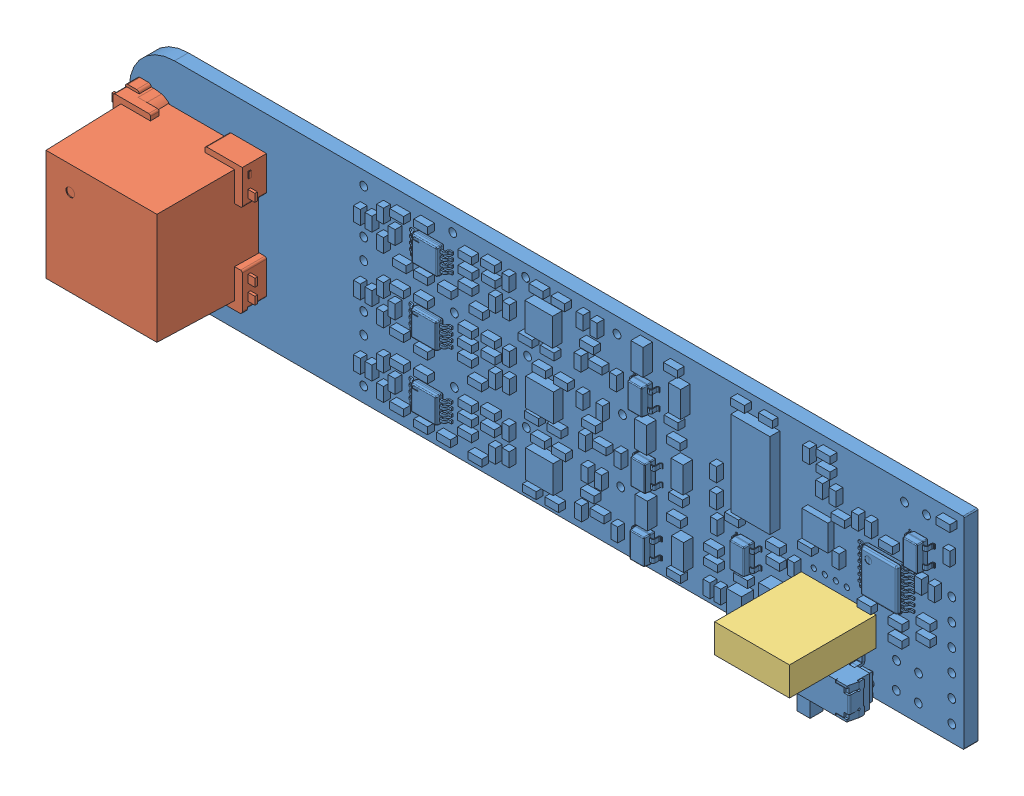
SolidWorks assembly rx_with_coil, configuration Default. Lengths in mm.
Overall size (96.32 25.78 13.35).
3 component instances, 3 part files, 8 mates.
Components (placement in the parent):
- RX_V0.9.step-1: RX_V0.9.step [Default] at (-81.31 -20.8269 7.6282) size (96.32 25.78 5.12)
- 3DCC08-1: 3DCC08 [Default] at (-62.3652 18.6935 13.4782) x (0 -1 0) z (-1 0 0) size (15 11.75 16.5)
- Part24^rx_with_coil-1: Part24^rx_with_coil [Default] at (-81.31 -20.8269 7.6282) size (8.63 3.31 10) (virtual)
Mates (geometry in assembly coordinates):
- Coincident1: coincident anti-aligned: plane of RX_V0.9.step-1 through (-65.689 6.4011 7.6282) normal (0 0 1); plane of 3DCC08-1 through (-62.3652 18.6935 7.6282) normal (0 0 -1)
- Parallel3: parallel aligned: line of RX_V0.9.step-1 through (-70.896 11.5581 7.6282) axis (0 1 0); line of 3DCC08-1 through (-55.7645 15.5435 7.8782) axis (0 1 0)
- Distance2: distance = 1.7808 mm: line of RX_V0.9.step-1 through (-70.896 11.5581 7.6282) axis (0 1 0); line of 3DCC08-1 through (-69.1152 25.1835 7.6282) axis (0 -1 0)
- Distance3: distance = 4.5106 mm: line of RX_V0.9.step-1 through (-65.689 29.6941 7.6282) axis (1 0 0); line of 3DCC08-1 through (-67.4302 25.1835 7.6282) axis (-1 0 0)
- InPlace1: in place: plane of ? through (-65.689 6.4011 7.6282) normal (0 0 1); plane of ? through (0 0 7.6282) normal (0 0 1); moOrthogonalPlaneRef_w of ? through (-65.689 6.4011 7.6282) normal (0 0 1); plane of ? through (0 0 7.6282) normal (0 1 0); plane of ? through (-65.689 6.4011 7.6282) normal (0 0 1); plane of ? through (0 0 7.6282) normal (1 0 0); plane of ? through (-65.689 6.4011 7.6282) normal (0 0 1); unknown of ?
- Coincident7: coincident aligned: plane of RX_V0.9.step-1 through (-65.689 6.4011 7.6282) normal (0 0 1); plane of Part24^rx_with_coil-1 through (-81.31 -20.8269 7.6282) normal (0 0 1)
- Coincident8: coincident aligned: moOrthogonalPlaneRef_w of RX_V0.9.step-1 through (-81.31 -20.8269 7.6282) normal (0 1 0); plane of Part24^rx_with_coil-1 through (-81.31 -20.8269 7.6282) normal (0 1 0)
- Coincident9: coincident anti-aligned: moOrthogonalPlaneRef_w of RX_V0.9.step-1 through (-81.31 -20.8269 7.6282) normal (-1 0 0); plane of Part24^rx_with_coil-1 through (-81.31 -20.8269 7.6282) normal (1 0 0)
